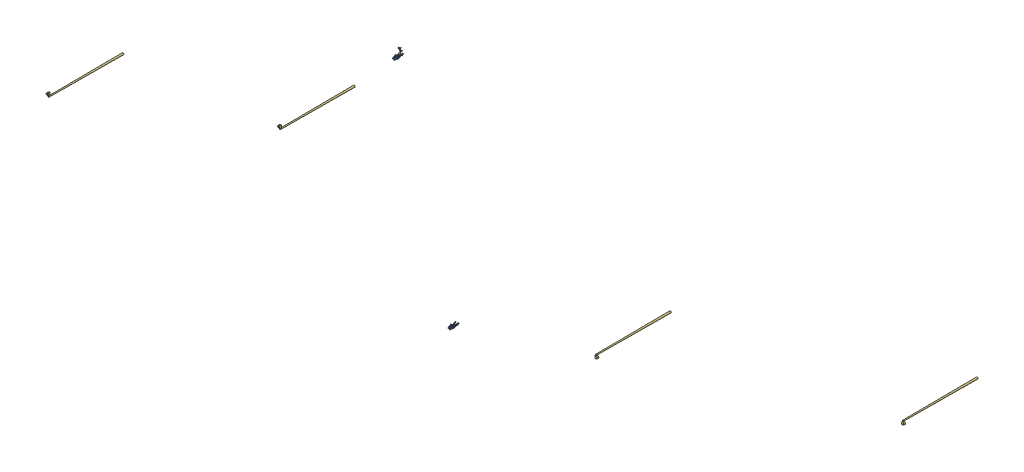
SolidWorks assembly Park scene, configuration Default. Lengths in mm.
Overall size (172997.33 43478.76 15155.93).
7 component instances, 3 part files, 8 mates.
Components (placement in the parent):
- Couple Walking v2-1: Couple Walking v2 [Default] at (90041.7631 17998.2932 0) size (971.22 682.9 1718.91)
- Couple Walking v2-2: Couple Walking v2 [Default] at (78840.4069 59479.1445 0) size (971.22 682.9 1718.91)
- German Shepherd-1: German Shepherd [Predeterminado] at (78938.2467 60181.5258 -995.4825) x (-0.927424 -0.373877 -0.010044) z (-0.373704 0.927415 -0.015684) size (212.95 642.55 996.13)
- LightPole-1: LightPole [Default] at (22635.286 31390.4456 0) x (-0.361809 0.932252 0) z (0 0 1) size (771.46 400 15150.67)
- LightPole-2: LightPole [Default] at (69285.9057 49048.0785 0) x (-0.361809 0.932252 0) z (0 0 1) size (771.46 400 15150.67)
- LightPole-3: LightPole [Default] at (133048.7527 41507.2409 0) x (0.217287 -0.976108 0) z (0 0 1) size (771.46 400 15150.67)
- LightPole-4: LightPole [Default] at (194905.5352 60880.401 0) x (0.217287 -0.976108 0) z (0 0 1) size (771.46 400 15150.67)
Mates (geometry in assembly coordinates):
- Coincident1: coincident anti-aligned: plane of Viaduct-1 through (121720.7023 -158145.4536 0) normal (0 0 -1)
- Coincident3: coincident: point of Viaduct-1
- Parallel1: parallel anti-aligned: plane of Viaduct-1 through (127159.1693 53321.2792 3923.6765) normal (0 -1 0)
- Coincident5: coincident aligned: plane of Couple Walking v2-1 through (90041.7631 17998.2932 0) normal (0 0 1)
- Coincident6: coincident aligned: plane of Couple Walking v2-2 through (78840.4069 59479.1445 0) normal (0 0 1)
- Tangent3: tangent anti-aligned: plane of Couple Walking v2-2 through (78840.4069 59479.1445 0) normal (0 0 1); face of German Shepherd-1
- Coincident7: coincident aligned: plane of LightPole-1 through (22635.286 31390.4456 0) normal (0 0 1)
- Coincident14: coincident aligned: plane of LightPole-3 through (133048.7527 41507.2409 0) normal (0 0 1)
